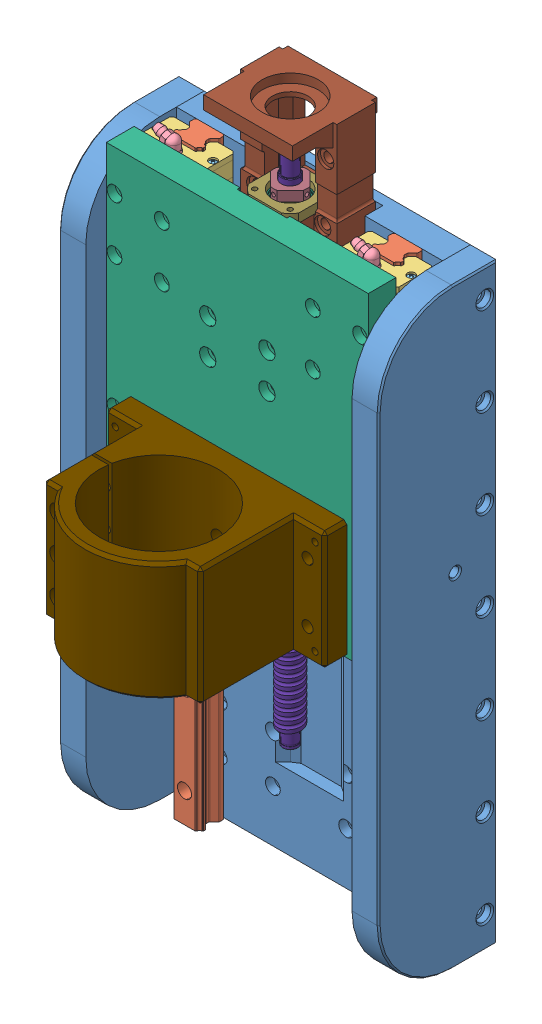
SolidWorks assembly Reverse_Z_Axis_x_slider, configuration Default. Lengths in mm.
Overall size (216 469 214.55).
80 component instances, 19 part files, 52 mates.
Components (placement in the parent):
- reverse_Z_Axis_Plate-1: reverse_Z_Axis_Plate [Default] at origin size (180 400 18.75)
- HGR20R LINEAR GUIDE RAIL, CONFIGURABLE-1: HGR20R LINEAR GUIDE RAIL, CONFIGURABLE [400 mm] at (67 -35 32.75) x (1 0 0) z (0 -1 0) size (20 17.5 400)
- HGH20CAZ0C-1: HGH20CAZ0C [Default] at (42.75 -4 -16) x (0 1 0) z (1 0 0) size (44 25.5 89.06)
  - HGH20CAZ0C, BLOCK, MIDSECTION-2: HGH20CAZ0C, BLOCK, MIDSECTION [Default] at origin size (44 25.5 77.5)
  - HGH20CAZ0C, BLOCK OIL FILLING PART-1: HGH20CAZ0C, BLOCK OIL FILLING PART [Default] at (0 11 33.75) x (0 0 -1) z (0 1 0) size (16.4 16.42 9.24)
  - HGH20CAZ0C, SCREW HEAD-1: HGH20CAZ0C, SCREW HEAD [Default] at (18.75 2.9 36.65) x (0 0 1) z (-1 0 0) size (2.26 5 5)
  - HGH20CAZ0C, SCREW HEAD-2: HGH20CAZ0C, SCREW HEAD [Default] at (-18.75 2.9 36.65) x (0 0 1) z (-1 0 0) size (2.26 5 5)
  - HGH20CAZ0C, SCREW HEAD-3: HGH20CAZ0C, SCREW HEAD [Default] at (18.75 2.9 -36.65) x (0 0 -1) z (1 0 0) size (2.26 5 5)
  - HGH20CAZ0C, SCREW HEAD-4: HGH20CAZ0C, SCREW HEAD [Default] at (-18.75 2.9 -36.65) x (0 0 -1) z (1 0 0) size (2.26 5 5)
- HGH20CAZ0C-5: HGH20CAZ0C [Default] at (-42.75 -184 -16) x (0 -1 0) z (-1 0 0) size (44 25.5 89.06)
  - HGH20CAZ0C, BLOCK, MIDSECTION-2: HGH20CAZ0C, BLOCK, MIDSECTION [Default] at origin size (44 25.5 77.5)
  - HGH20CAZ0C, BLOCK OIL FILLING PART-1: HGH20CAZ0C, BLOCK OIL FILLING PART [Default] at (0 11 33.75) x (0 0 -1) z (0 1 0) size (16.4 16.42 9.24)
  - HGH20CAZ0C, SCREW HEAD-1: HGH20CAZ0C, SCREW HEAD [Default] at (18.75 2.9 36.65) x (0 0 1) z (-1 0 0) size (2.26 5 5)
  - HGH20CAZ0C, SCREW HEAD-2: HGH20CAZ0C, SCREW HEAD [Default] at (-18.75 2.9 36.65) x (0 0 1) z (-1 0 0) size (2.26 5 5)
  - HGH20CAZ0C, SCREW HEAD-3: HGH20CAZ0C, SCREW HEAD [Default] at (18.75 2.9 -36.65) x (0 0 -1) z (1 0 0) size (2.26 5 5)
  - HGH20CAZ0C, SCREW HEAD-4: HGH20CAZ0C, SCREW HEAD [Default] at (-18.75 2.9 -36.65) x (0 0 -1) z (1 0 0) size (2.26 5 5)
- HGH20CAZ0C-6: HGH20CAZ0C [Default] at (67.0186 124.2015 32.7963) x (-1 0 0) z (0 1 0) size (44 25.5 89.06)
  - HGH20CAZ0C, BLOCK, MIDSECTION-2: HGH20CAZ0C, BLOCK, MIDSECTION [Default] at origin size (44 25.5 77.5)
  - HGH20CAZ0C, BLOCK OIL FILLING PART-1: HGH20CAZ0C, BLOCK OIL FILLING PART [Default] at (0 11 33.75) x (0 0 -1) z (0 1 0) size (16.4 16.42 9.24)
  - HGH20CAZ0C, SCREW HEAD-1: HGH20CAZ0C, SCREW HEAD [Default] at (18.75 2.9 36.65) x (0 0 1) z (-1 0 0) size (2.26 5 5)
  - HGH20CAZ0C, SCREW HEAD-2: HGH20CAZ0C, SCREW HEAD [Default] at (-18.75 2.9 36.65) x (0 0 1) z (-1 0 0) size (2.26 5 5)
  - HGH20CAZ0C, SCREW HEAD-3: HGH20CAZ0C, SCREW HEAD [Default] at (18.75 2.9 -36.65) x (0 0 -1) z (1 0 0) size (2.26 5 5)
  - HGH20CAZ0C, SCREW HEAD-4: HGH20CAZ0C, SCREW HEAD [Default] at (-18.75 2.9 -36.65) x (0 0 -1) z (1 0 0) size (2.26 5 5)
- HGH20CAZ0C-7: HGH20CAZ0C [Default] at (67.0186 -0.9985 32.7963) x (-1 0 0) z (0 1 0) size (44 25.5 89.06)
  - HGH20CAZ0C, BLOCK, MIDSECTION-2: HGH20CAZ0C, BLOCK, MIDSECTION [Default] at origin size (44 25.5 77.5)
  - HGH20CAZ0C, BLOCK OIL FILLING PART-1: HGH20CAZ0C, BLOCK OIL FILLING PART [Default] at (0 11 33.75) x (0 0 -1) z (0 1 0) size (16.4 16.42 9.24)
  - HGH20CAZ0C, SCREW HEAD-1: HGH20CAZ0C, SCREW HEAD [Default] at (18.75 2.9 36.65) x (0 0 1) z (-1 0 0) size (2.26 5 5)
  - HGH20CAZ0C, SCREW HEAD-2: HGH20CAZ0C, SCREW HEAD [Default] at (-18.75 2.9 36.65) x (0 0 1) z (-1 0 0) size (2.26 5 5)
  - HGH20CAZ0C, SCREW HEAD-3: HGH20CAZ0C, SCREW HEAD [Default] at (18.75 2.9 -36.65) x (0 0 -1) z (1 0 0) size (2.26 5 5)
  - HGH20CAZ0C, SCREW HEAD-4: HGH20CAZ0C, SCREW HEAD [Default] at (-18.75 2.9 -36.65) x (0 0 -1) z (1 0 0) size (2.26 5 5)
- reverse_Z_Spindle_Plate-1: reverse_Z_Spindle_Plate [Default] at (0 103.0183 48.7963) size (177.04 220.5 18.75)
- HGH20CAZ0C-8: HGH20CAZ0C [Default] at (-42.75 -4 -16) x (0 -1 0) z (-1 0 0) size (44 25.5 89.06)
  - HGH20CAZ0C, BLOCK, MIDSECTION-2: HGH20CAZ0C, BLOCK, MIDSECTION [Default] at origin size (44 25.5 77.5)
  - HGH20CAZ0C, BLOCK OIL FILLING PART-1: HGH20CAZ0C, BLOCK OIL FILLING PART [Default] at (0 11 33.75) x (0 0 -1) z (0 1 0) size (16.4 16.42 9.24)
  - HGH20CAZ0C, SCREW HEAD-1: HGH20CAZ0C, SCREW HEAD [Default] at (18.75 2.9 36.65) x (0 0 1) z (-1 0 0) size (2.26 5 5)
  - HGH20CAZ0C, SCREW HEAD-2: HGH20CAZ0C, SCREW HEAD [Default] at (-18.75 2.9 36.65) x (0 0 1) z (-1 0 0) size (2.26 5 5)
  - HGH20CAZ0C, SCREW HEAD-3: HGH20CAZ0C, SCREW HEAD [Default] at (18.75 2.9 -36.65) x (0 0 -1) z (1 0 0) size (2.26 5 5)
  - HGH20CAZ0C, SCREW HEAD-4: HGH20CAZ0C, SCREW HEAD [Default] at (-18.75 2.9 -36.65) x (0 0 -1) z (1 0 0) size (2.26 5 5)
- HGR20R LINEAR GUIDE RAIL, CONFIGURABLE-2: HGR20R LINEAR GUIDE RAIL, CONFIGURABLE [400 mm] at (-67 -35 32.75) x (1 0 0) z (0 -1 0) size (20 17.5 400)
- HGH20CAZ0C-9: HGH20CAZ0C [Default] at (-67.0186 124.2015 32.7963) x (-1 0 0) z (0 1 0) size (44 25.5 89.06)
  - HGH20CAZ0C, BLOCK, MIDSECTION-2: HGH20CAZ0C, BLOCK, MIDSECTION [Default] at origin size (44 25.5 77.5)
  - HGH20CAZ0C, BLOCK OIL FILLING PART-1: HGH20CAZ0C, BLOCK OIL FILLING PART [Default] at (0 11 33.75) x (0 0 -1) z (0 1 0) size (16.4 16.42 9.24)
  - HGH20CAZ0C, SCREW HEAD-1: HGH20CAZ0C, SCREW HEAD [Default] at (18.75 2.9 36.65) x (0 0 1) z (-1 0 0) size (2.26 5 5)
  - HGH20CAZ0C, SCREW HEAD-2: HGH20CAZ0C, SCREW HEAD [Default] at (-18.75 2.9 36.65) x (0 0 1) z (-1 0 0) size (2.26 5 5)
  - HGH20CAZ0C, SCREW HEAD-3: HGH20CAZ0C, SCREW HEAD [Default] at (18.75 2.9 -36.65) x (0 0 -1) z (1 0 0) size (2.26 5 5)
  - HGH20CAZ0C, SCREW HEAD-4: HGH20CAZ0C, SCREW HEAD [Default] at (-18.75 2.9 -36.65) x (0 0 -1) z (1 0 0) size (2.26 5 5)
- HGH20CAZ0C-10: HGH20CAZ0C [Default] at (-67.0186 -0.9985 32.7963) x (-1 0 0) z (0 1 0) size (44 25.5 89.06)
  - HGH20CAZ0C, BLOCK, MIDSECTION-2: HGH20CAZ0C, BLOCK, MIDSECTION [Default] at origin size (44 25.5 77.5)
  - HGH20CAZ0C, BLOCK OIL FILLING PART-1: HGH20CAZ0C, BLOCK OIL FILLING PART [Default] at (0 11 33.75) x (0 0 -1) z (0 1 0) size (16.4 16.42 9.24)
  - HGH20CAZ0C, SCREW HEAD-1: HGH20CAZ0C, SCREW HEAD [Default] at (18.75 2.9 36.65) x (0 0 1) z (-1 0 0) size (2.26 5 5)
  - HGH20CAZ0C, SCREW HEAD-2: HGH20CAZ0C, SCREW HEAD [Default] at (-18.75 2.9 36.65) x (0 0 1) z (-1 0 0) size (2.26 5 5)
  - HGH20CAZ0C, SCREW HEAD-3: HGH20CAZ0C, SCREW HEAD [Default] at (18.75 2.9 -36.65) x (0 0 -1) z (1 0 0) size (2.26 5 5)
  - HGH20CAZ0C, SCREW HEAD-4: HGH20CAZ0C, SCREW HEAD [Default] at (-18.75 2.9 -36.65) x (0 0 -1) z (1 0 0) size (2.26 5 5)
- HGH20CAZ0C-11: HGH20CAZ0C [Default] at (42.75 -184 -16) x (0 1 0) z (1 0 0) size (44 25.5 89.06)
  - HGH20CAZ0C, BLOCK, MIDSECTION-2: HGH20CAZ0C, BLOCK, MIDSECTION [Default] at origin size (44 25.5 77.5)
  - HGH20CAZ0C, BLOCK OIL FILLING PART-1: HGH20CAZ0C, BLOCK OIL FILLING PART [Default] at (0 11 33.75) x (0 0 -1) z (0 1 0) size (16.4 16.42 9.24)
  - HGH20CAZ0C, SCREW HEAD-1: HGH20CAZ0C, SCREW HEAD [Default] at (18.75 2.9 36.65) x (0 0 1) z (-1 0 0) size (2.26 5 5)
  - HGH20CAZ0C, SCREW HEAD-2: HGH20CAZ0C, SCREW HEAD [Default] at (-18.75 2.9 36.65) x (0 0 1) z (-1 0 0) size (2.26 5 5)
  - HGH20CAZ0C, SCREW HEAD-3: HGH20CAZ0C, SCREW HEAD [Default] at (18.75 2.9 -36.65) x (0 0 -1) z (1 0 0) size (2.26 5 5)
  - HGH20CAZ0C, SCREW HEAD-4: HGH20CAZ0C, SCREW HEAD [Default] at (-18.75 2.9 -36.65) x (0 0 -1) z (1 0 0) size (2.26 5 5)
- x-axis-ballnut-1: x-axis-ballnut [Default] at (-179.8948 -22.7662 -174.6595) x (0 1 0) z (1 0 0) size (52 44 50)
  - Nut_block_spacer-1: Nut_block_spacer [Default] at (-71.2338 174.6595 184.8948) x (1 0 0) z (0 -1 0) size (52 40 4)
  - SFU Ball Nut-1: SFU Ball Nut [1605-3] at (-71.2338 150.6595 234.8948) size (48 40 43)
  - DSG16H Ball Nut Housing-1: DSG16H Ball Nut Housing [Default] at (-71.2338 150.6595 224.8948) x (1 0 0) z (0 1 0) size (52 40 40)
- z-axis-ballnut-1: z-axis-ballnut [Default] at (-186.6152 33.6223 200.6714) x (0 -1 0) z (1 0 0) size (50 40 52)
  - DSG16H Ball Nut Housing_thinned-1: DSG16H Ball Nut Housing_thinned [Default] at (-76.396 168.875 186.6152) x (0 0 -1) z (0 -1 0) size (52 40 34)
  - SFU Ball Nut-1: SFU Ball Nut [1605-3] at (-86.396 168.875 186.6152) x (0 0 1) z (-1 0 0) size (48 40 43)
- BJ12-1: BJ12 [Default] at (32.5 140 6.7963) x (0 1 0) z (1 0 0) size (83.5 57 65)
  - _____^1728663652539-1: _____^1728663652539 [Default] at origin size (83 57 65)
  - __^1728663652539_3-1: __^1728663652539_3 [Default] at (22.7 25 -32.5) x (0 -1 0) z (1 0 0) size (34 34 7.38)
  - ____^1728663652539-1: ____^1728663652539 [Default] at (27.5025 25 -32.5) x (0 0 -1) z (1 0 0) size (22.8 22.8 7.78)
  - __^1728663652539-1: __^1728663652539 [Default] at (17.1687 25 -32.5) x (0 0 -1) z (1 0 0) size (25.5 25.5 16.23)
  - __^1728663652539_2-1: __^1728663652539_2 [Default] at (2 25 -32.5) x (0 0 -1) z (1 0 0) size (23.8 23.8 3)
  - ___^1728663652539-1: ___^1728663652539 [Default] at (5 25 -32.5) x (0 0.017502 0.999847) z (-1 0 0) size (18 18 5.5)
  - __^1728663652539_2-2: __^1728663652539_2 [Default] at (24.225 25 -32.5) x (0 0.924225 0.381849) z (-1 0 0) size (23.8 23.8 3)
  - ___^1728663652539-2: ___^1728663652539 [Default] at (26.725 25 -32.5) x (0 0 1) z (-1 0 0) size (18 18 5.5)
- Generic Ballscrew_zaxis-1: Generic Ballscrew_zaxis [SFU-1605] at (0 193.5 31.7963) x (0 0 1) z (0 1 0) size (16.11 16 350)
- 80_mmSpinde_Bracket_part-1: 80_mmSpinde_Bracket_part [Default] at (192.745 -18.9551 14.3463) x (1 0 0) z (0 1 0) size (148 103 80)
- Z_axis_assembly_wing_long-1: Z_axis_assembly_wing_long [Default] at (90 36 -1) x (0 0 1) z (1 0 0) size (81 411 18)
- Z_axis_assembly_wing_long-2: Z_axis_assembly_wing_long [Default] at (-90 -106 -1) x (0 0 1) z (-1 0 0) size (81 411 18)
Mates (geometry in assembly coordinates):
- Coincident1: coincident anti-aligned: plane of reverse_Z_Axis_Plate-1 through (0 0 18.75) normal (0 0 1); plane of HGR20R LINEAR GUIDE RAIL, CONFIGURABLE-1 through (58 -235 18.75) normal (0 0 -1)
- Distance1: distance = 0 mm aligned: plane of HGR20R LINEAR GUIDE RAIL, CONFIGURABLE-1 through (58 -235 22.4115) normal (0 -1 0); plane of reverse_Z_Axis_Plate-1 through (-90 -235 18.75) normal (0 -1 0)
- Distance2: distance = 13 mm aligned: plane of HGR20R LINEAR GUIDE RAIL, CONFIGURABLE-1 through (77 -235 22.4115) normal (1 0 0); plane of reverse_Z_Axis_Plate-1 through (90 165 18.75) normal (1 0 0)
- Coincident2: coincident anti-aligned: plane of reverse_Z_Axis_Plate-1 through (0 0 0) normal (0 0 -1); plane of HGH20CAZ0C-1/HGH20CAZ0C, BLOCK, MIDSECTION-2 through (68 -25 0) normal (0 0 1)
- Concentric1: concentric aligned: cylinder of reverse_Z_Axis_Plate-1 through (24.75 12 18.75) axis (0 0 1) radius 2.75; cylinder of HGH20CAZ0C-1/HGH20CAZ0C, BLOCK, MIDSECTION-2 through (24.75 12 0) axis (0 0 1) radius 2.1
- Parallel2: parallel aligned: plane of reverse_Z_Axis_Plate-1 through (90 165 18.75) normal (1 0 0); plane of HGH20CAZ0C-1/HGH20CAZ0C, BLOCK, MIDSECTION-2 through (81.5 -13.8292 -19.1926) normal (1 0 0)
- Coincident16: coincident anti-aligned: plane of reverse_Z_Axis_Plate-1 through (0 0 0) normal (0 0 -1); plane of HGH20CAZ0C-5/HGH20CAZ0C, BLOCK, MIDSECTION-2 through (-68 -205 0) normal (0 0 1)
- Concentric2: concentric aligned: cylinder of reverse_Z_Axis_Plate-1 through (-60.75 -200 18.75) axis (0 0 1) radius 2.75; cylinder of HGH20CAZ0C-5/HGH20CAZ0C, BLOCK, MIDSECTION-2 through (-60.75 -200 0) axis (0 0 1) radius 2.1
- Concentric3: concentric aligned: cylinder of reverse_Z_Axis_Plate-1 through (-24.75 -168 18.75) axis (0 0 1) radius 2.75; cylinder of HGH20CAZ0C-5/HGH20CAZ0C, BLOCK, MIDSECTION-2 through (-24.75 -168 0) axis (0 0 1) radius 2.1
- Concentric5: concentric anti-aligned: cylinder of HGR20R LINEAR GUIDE RAIL, CONFIGURABLE-1 through (57.1894 -235 29.6037) axis (0 1 0) radius 2; cylinder of HGH20CAZ0C-6/HGH20CAZ0C, BLOCK, MIDSECTION-2 through (57.1894 149.4515 29.6037) axis (0 -1 0) radius 2.13
- Parallel4: parallel anti-aligned: plane of HGR20R LINEAR GUIDE RAIL, CONFIGURABLE-1 through (74.2357 -235 36.25) normal (0 0 1); plane of HGH20CAZ0C-6/HGH20CAZ0C, BLOCK, MIDSECTION-2 through (74.3186 149.4515 36.2963) normal (0 0 -1)
- Concentric6: concentric anti-aligned: cylinder of HGR20R LINEAR GUIDE RAIL, CONFIGURABLE-1 through (57.1894 -235 29.6037) axis (0 1 0) radius 2; cylinder of HGH20CAZ0C-7/HGH20CAZ0C, BLOCK, MIDSECTION-2 through (57.1894 34.2515 29.6037) axis (0 -1 0) radius 2.13
- Parallel5: parallel anti-aligned: plane of HGR20R LINEAR GUIDE RAIL, CONFIGURABLE-1 through (74.2357 -235 36.25) normal (0 0 1); plane of HGH20CAZ0C-7/HGH20CAZ0C, BLOCK, MIDSECTION-2 through (74.3186 24.2515 36.2963) normal (0 0 -1)
- Distance3: distance = 85 mm: cylinder of HGH20CAZ0C-6/HGH20CAZ0C, BLOCK, MIDSECTION-2 through (83.0186 106.2015 48.7963) axis (0 0 1) radius 2.1; cylinder of HGH20CAZ0C-7/HGH20CAZ0C, BLOCK, MIDSECTION-2 through (83.0186 17.0015 48.7963) axis (0 0 1) radius 2.1
- Concentric8: concentric anti-aligned: cylinder of HGH20CAZ0C-6/HGH20CAZ0C, BLOCK, MIDSECTION-2 through (83.0186 142.2015 48.7963) axis (0 0 1) radius 2.1; cylinder of reverse_Z_Spindle_Plate-1 through (83.0186 142.2015 67.5463) axis (0 0 -1) radius 3
- Concentric9: concentric anti-aligned: cylinder of HGH20CAZ0C-6/HGH20CAZ0C, BLOCK, MIDSECTION-2 through (83.0186 106.2015 48.7963) axis (0 0 1) radius 2.1; cylinder of reverse_Z_Spindle_Plate-1 through (83.0186 106.2015 67.5463) axis (0 0 -1) radius 3
- Coincident18: coincident anti-aligned: plane of HGH20CAZ0C-6/HGH20CAZ0C, BLOCK, MIDSECTION-2 through (46.0186 149.4515 48.7963) normal (0 0 1); plane of reverse_Z_Spindle_Plate-1 through (0 103.0183 48.7963) normal (0 0 -1)
- Coincident19: coincident anti-aligned: plane of reverse_Z_Axis_Plate-1 through (0 0 0) normal (0 0 -1); plane of HGH20CAZ0C-8/HGH20CAZ0C, BLOCK, MIDSECTION-2 through (-68 -25 0) normal (0 0 1)
- Concentric10: concentric aligned: cylinder of reverse_Z_Axis_Plate-1 through (-60.75 -20 18.75) axis (0 0 1) radius 2.75; cylinder of HGH20CAZ0C-8/HGH20CAZ0C, BLOCK, MIDSECTION-2 through (-60.75 -20 0) axis (0 0 1) radius 2.1
- Concentric11: concentric aligned: cylinder of reverse_Z_Axis_Plate-1 through (-24.75 12 18.75) axis (0 0 1) radius 2.75; cylinder of HGH20CAZ0C-8/HGH20CAZ0C, BLOCK, MIDSECTION-2 through (-24.75 12 0) axis (0 0 1) radius 2.1
- Distance4: distance = 13 mm aligned: plane of HGR20R LINEAR GUIDE RAIL, CONFIGURABLE-2 through (-77 -235 22.4115) normal (-1 0 0); plane of reverse_Z_Axis_Plate-1 through (-90 -235 18.75) normal (-1 0 0)
- Coincident21: coincident anti-aligned: plane of reverse_Z_Axis_Plate-1 through (0 0 18.75) normal (0 0 1); plane of HGR20R LINEAR GUIDE RAIL, CONFIGURABLE-2 through (-76 -235 18.75) normal (0 0 -1)
- Coincident22: coincident aligned: plane of reverse_Z_Axis_Plate-1 through (-90 165 18.75) normal (0 1 0); plane of HGR20R LINEAR GUIDE RAIL, CONFIGURABLE-2 through (-76 165 22.4115) normal (0 1 0)
- Coincident23: coincident anti-aligned: plane of reverse_Z_Spindle_Plate-1 through (0 103.0183 48.7963) normal (0 0 -1); plane of HGH20CAZ0C-9/HGH20CAZ0C, BLOCK, MIDSECTION-2 through (-46.0186 149.4515 48.7963) normal (0 0 1)
- Concentric12: concentric anti-aligned: cylinder of reverse_Z_Spindle_Plate-1 through (-83.0186 142.2015 67.5463) axis (0 0 -1) radius 3; cylinder of HGH20CAZ0C-9/HGH20CAZ0C, BLOCK, MIDSECTION-2 through (-83.0186 142.2015 48.7963) axis (0 0 1) radius 2.1
- Concentric13: concentric anti-aligned: cylinder of reverse_Z_Spindle_Plate-1 through (-51.0186 106.2015 67.5463) axis (0 0 -1) radius 3; cylinder of HGH20CAZ0C-9/HGH20CAZ0C, BLOCK, MIDSECTION-2 through (-51.0186 106.2015 48.7963) axis (0 0 1) radius 2.1
- Coincident24: coincident anti-aligned: plane of reverse_Z_Spindle_Plate-1 through (0 103.0183 48.7963) normal (0 0 -1); plane of HGH20CAZ0C-10/HGH20CAZ0C, BLOCK, MIDSECTION-2 through (-46.0186 24.2515 48.7963) normal (0 0 1)
- Concentric14: concentric anti-aligned: cylinder of reverse_Z_Spindle_Plate-1 through (-83.0186 -18.9985 67.5463) axis (0 0 -1) radius 3; cylinder of HGH20CAZ0C-10/HGH20CAZ0C, BLOCK, MIDSECTION-2 through (-83.0186 -18.9985 48.7963) axis (0 0 1) radius 2.1
- Concentric15: concentric anti-aligned: cylinder of reverse_Z_Spindle_Plate-1 through (-51.0186 17.0015 67.5463) axis (0 0 -1) radius 3; cylinder of HGH20CAZ0C-10/HGH20CAZ0C, BLOCK, MIDSECTION-2 through (-51.0186 17.0015 48.7963) axis (0 0 1) radius 2.1
- Coincident25: coincident anti-aligned: plane of reverse_Z_Axis_Plate-1 through (0 0 0) normal (0 0 -1); plane of HGH20CAZ0C-11/HGH20CAZ0C, BLOCK, MIDSECTION-2 through (68 -163 0) normal (0 0 1)
- Concentric16: concentric aligned: cylinder of reverse_Z_Axis_Plate-1 through (24.75 -200 18.75) axis (0 0 1) radius 2.75; cylinder of HGH20CAZ0C-11/HGH20CAZ0C, BLOCK, MIDSECTION-2 through (24.75 -200 0) axis (0 0 1) radius 2.1
- Concentric17: concentric aligned: cylinder of reverse_Z_Axis_Plate-1 through (24.75 -168 18.75) axis (0 0 1) radius 2.75; cylinder of HGH20CAZ0C-11/HGH20CAZ0C, BLOCK, MIDSECTION-2 through (24.75 -168 0) axis (0 0 1) radius 2.1
- Coincident27: coincident anti-aligned: plane of reverse_Z_Axis_Plate-1 through (0 0 0) normal (0 0 -1); plane of x-axis-ballnut-1/Nut_block_spacer-1 through (5 -94 0) normal (0 0 1)
- Distance5: distance = 42 mm anti-aligned: plane of x-axis-ballnut-1/Nut_block_spacer-1 through (6 -68 -4) normal (0 1 0); plane of HGH20CAZ0C-1/HGH20CAZ0C, BLOCK, MIDSECTION-2 through (68 -26 -1) normal (0 -1 0)
- Distance6: distance = 45 mm aligned: plane of reverse_Z_Axis_Plate-1 through (90 165 18.75) normal (1 0 0); plane of x-axis-ballnut-1/Nut_block_spacer-1 through (45 -119 -4) normal (1 0 0)
- Coincident31: coincident anti-aligned: plane of reverse_Z_Spindle_Plate-1 through (0 103.0183 48.7963) normal (0 0 -1); plane of z-axis-ballnut-1/DSG16H Ball Nut Housing_thinned-1 through (0 110.0183 48.7963) normal (0 0 1)
- Concentric21: concentric aligned: cylinder of reverse_Z_Spindle_Plate-1 through (-20 102.0183 67.5463) axis (0 0 1) radius 3; cylinder of z-axis-ballnut-1/DSG16H Ball Nut Housing_thinned-1 through (-20 102.0183 28.3111) axis (0 0 1) radius 3
- Concentric23: concentric aligned: cylinder of reverse_Z_Spindle_Plate-1 through (20 78.0183 67.5463) axis (0 0 1) radius 3; cylinder of z-axis-ballnut-1/DSG16H Ball Nut Housing_thinned-1 through (20 78.0183 28.3111) axis (0 0 1) radius 3
- Parallel9: parallel anti-aligned: plane of reverse_Z_Axis_Plate-1 through (0 0 18.75) normal (0 0 1); plane of BJ12-1/_____^1728663652539-1 through (32.5 223 6.7963) normal (0 0 -1)
- Concentric25: concentric aligned: cylinder of BJ12-1/____^1728663652539-1 through (0 167.5015 31.7963) axis (0 1 0) radius 5.16; cylinder of Generic Ballscrew_zaxis-1 through (0 210.5125 31.7963) axis (0 1 0) radius 5
- Coincident35: coincident anti-aligned: plane of BJ12-1/___^1728663652539-1 through (0 139.5 31.7963) normal (0 -1 0); plane of Generic Ballscrew_zaxis-1 through (6 139.5 31.7963) normal (0 1 0)
- Concentric26: concentric aligned: cylinder of reverse_Z_Axis_Plate-1 through (23 146 0) axis (0 0 1) radius 2.5; cylinder of BJ12-1/_____^1728663652539-1 through (23 146 3.2953) axis (0 0 1) radius 3.3
- Concentric27: concentric aligned: cylinder of reverse_Z_Axis_Plate-1 through (-23 159 0) axis (0 0 1) radius 2.5; cylinder of BJ12-1/_____^1728663652539-1 through (-23 159 3.2953) axis (0 0 1) radius 3.3
- Coincident40: coincident anti-aligned: plane of reverse_Z_Spindle_Plate-1 through (0 103.0183 67.5463) normal (0 0 1); plane of 80_mmSpinde_Bracket_part-1 through (-74.0014 28.9515 67.5463) normal (0 0 -1)
- Coincident41: coincident aligned: plane of reverse_Z_Spindle_Plate-1 through (-88.5186 -51.0485 67.5463) normal (0 -1 0); plane of 80_mmSpinde_Bracket_part-1 through (-0.0014 -51.0485 120.5463) normal (0 -1 0)
- Distance8: distance = 14.52 mm aligned: plane of 80_mmSpinde_Bracket_part-1 through (73.9986 28.9515 67.5463) normal (1 0 0); plane of reverse_Z_Spindle_Plate-1 through (88.5186 149.4515 67.5463) normal (1 0 0)
- Coincident44: coincident anti-aligned: plane of reverse_Z_Axis_Plate-1 through (90 165 18.75) normal (1 0 0); plane of Z_axis_assembly_wing_long-1 through (90 36 -1) normal (-1 0 0)
- Coincident45: coincident aligned: plane of reverse_Z_Axis_Plate-1 through (-90 -235 18.75) normal (0 -1 0); plane of Z_axis_assembly_wing_long-1 through (108 -235 0) normal (0 -1 0)
- Coincident46: coincident aligned: plane of reverse_Z_Axis_Plate-1 through (0 0 0) normal (0 0 -1); plane of Z_axis_assembly_wing_long-1 through (108 -235 0) normal (0 0 -1)
- Coincident47: coincident anti-aligned: plane of reverse_Z_Axis_Plate-1 through (-90 -235 18.75) normal (-1 0 0); plane of Z_axis_assembly_wing_long-2 through (-90 -106 -1) normal (1 0 0)
- Coincident48: coincident aligned: plane of reverse_Z_Axis_Plate-1 through (-90 -235 18.75) normal (0 -1 0); plane of Z_axis_assembly_wing_long-2 through (-108 -235 0) normal (0 -1 0)
- Coincident49: coincident aligned: plane of reverse_Z_Axis_Plate-1 through (0 0 0) normal (0 0 -1); plane of Z_axis_assembly_wing_long-2 through (-108 165 0) normal (0 0 -1)
